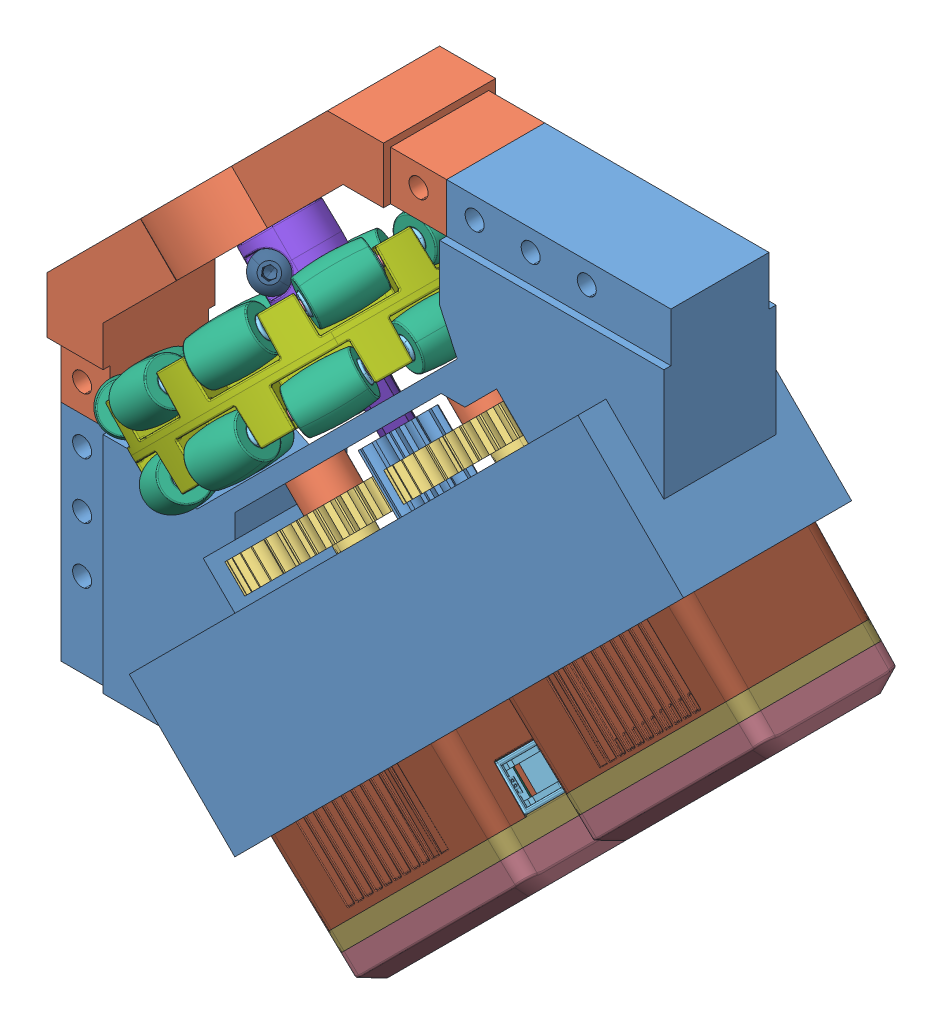
SolidWorks assembly HoloModuleAssemly1, configuration Default. Lengths in mm.
Overall size (169.7 169.56 123.95).
151 component instances, 28 part files, 46 mates.
Components (placement in the parent):
- Motor Bracket-1: Motor Bracket [Default] at (-26.4665 163.4033 98.185) size (148.89 148.89 38.1)
- Wheel Bracket-1: Wheel Bracket [Default] at (-26.4665 163.4033 98.185) size (88.9 88.9 38.1)
- Holo_Motor_Shaft-1: Holo_Motor_Shaft [Default] at (163.1236 9.787 110.8958) x (0.619089 0.619089 -0.483174) z (0.707107 -0.707107 0) size (3.28 3.28 30.48)
- Holo_Motor_Shaft-2: Holo_Motor_Shaft [Default] at (127.2026 -26.134 110.8958) x (-0.341656 -0.341656 -0.875524) z (0.707107 -0.707107 0) size (3.28 3.28 30.48)
- V5 Smart Motor (276-4840) no cap-1: V5 Smart Motor (276-4840) no cap [Default] at (47.4004 35.6548 110.885) x (0.707107 0.707107 0) z (-0.707107 0.707107 0) size (59.01 35.33 59.91)
  - V5 Smart Motor (276-4840).step-1: V5 Smart Motor (276-4840).step [Default] at origin size (59.01 35.33 59.91)
    - 276-4840-900 Rev6_Instruction.step-1: 276-4840-900 Rev6_Instruction.step [Default] at (-14.3 0 -17.2) size (52.79 15.94 38.15)
      - 276-4840-901 Rev6.step-1: 276-4840-901 Rev6.step [Default] at (10.75 -10.05 17.8) x (-1 0 0) z (0 0 1) size (49.9 1.6 38.15)
      - 276-4840-902 Rev2.step-1: 276-4840-902 Rev2.step [Default] at (31.25 -9.25 6.2) x (0 0 -1) z (0 -1 0) size (10.35 11.39 15.94)
      - 276-4840-022 Rev4.step-1: 276-4840-022 Rev4.step [Default] at (31.25 -9.25 6.2) x (0 0 -1) z (1 0 0) size (10.26 9.1 5.51)
    - 276-4840-110 Rev10_Instruction.step-1: 276-4840-110 Rev10_Instruction.step [Default] at (12.7 0 14.7) size (35.33 35.33 31.1)
      - 276-4840-061 Rev7_Ring_Gear_Fixed01 .6 Rev3.step-1: 276-4840-061 Rev7_Ring_Gear_Fixed01 .6 Rev3.step [Default] at origin size (28.79 28.39 24.6)
      - 276-4840-018 Rev6.step-1: 276-4840-018 Rev6.step [Default] at (0 0 6.7) x (-0.483174 0.875524 0) z (0 0 1) size (26 26 12.3)
      - 276-4840-059 Rev2.step-1: 276-4840-059 Rev2.step [Default] at (0 0 10.3) size (28.4 28.4 8.5)
      - 276-4840-062 Rev1.step-1: 276-4840-062 Rev1.step [Default] at (-12.1353 8.8168 12.3) x (0.956835 -0.290632 0) z (-0.290632 -0.956835 0) size (3.2 6.56 3.2)
      - 276-4840-062 Rev1.step-2: 276-4840-062 Rev1.step [Default] at (12.1353 8.8168 12.3) x (0.978427 0.206591 0) z (0.206591 -0.978427 0) size (3.2 6.56 3.2)
      - 276-4840-062 Rev1.step-3: 276-4840-062 Rev1.step [Default] at (-12.1353 -8.8168 12.3) x (0.72563 0.688086 0) z (0.688086 -0.72563 0) size (3.2 6.56 3.2)
    - 276-4840-001 Rev38.step-1: 276-4840-001 Rev38.step [Default] at origin size (57.3 33 46.9)
    - 276-4840-005 Rev27.step-1: 276-4840-005 Rev27.step [Default] at (0 0 -17.95) size (56.17 31.87 12.9)
    - 276-4840-004 Rev16.step-1: 276-4840-004 Rev16.step [Default] at (0 0 -19.2) size (56.01 31.71 9.21)
    - 276-4840-009 Rev3.step-1: 276-4840-009 Rev3.step [Default] at (25.45 13.5 15.7) x (0.19987 -0.979823 0) z (-0.979823 -0.19987 0) size (3.4 41.31 4.34)
    - 276-4840-009 Rev3.step-2: 276-4840-009 Rev3.step [Default] at (-25.45 -13.5 15.7) x (-0.998855 0.047836 0) z (0.047836 0.998855 0) size (3.4 41.31 4.34)
    - 276-4840-009 Rev3.step-3: 276-4840-009 Rev3.step [Default] at (25.45 -13.5 15.7) x (-0.975374 0.220559 0) z (0.220559 0.975374 0) size (3.4 41.31 4.34)
    - 276-4840-009 Rev3.step-4: 276-4840-009 Rev3.step [Default] at (-25.45 13.5 15.7) x (-0.922256 0.38658 0) z (0.38658 0.922256 0) size (3.4 41.31 4.34)
    - 276-4840-025 Rev19.step-1: 276-4840-025 Rev19.step [Default] at (12.7 0 -22.63) x (-0.993315 0.115437 0) z (0 0 1) size (14.82 14.83 35.18)
- V5 Smart Motor (276-4840) no cap-2: V5 Smart Motor (276-4840) no cap [Default] at (101.282 89.5364 110.885) x (-0.707107 -0.707107 0) z (-0.707107 0.707107 0) size (59.01 35.33 59.91)
  - V5 Smart Motor (276-4840).step-1: V5 Smart Motor (276-4840).step [Default] at origin size (59.01 35.33 59.91)
    - 276-4840-900 Rev6_Instruction.step-1: 276-4840-900 Rev6_Instruction.step [Default] at (-14.3 0 -17.2) size (52.79 15.94 38.15)
      - 276-4840-901 Rev6.step-1: 276-4840-901 Rev6.step [Default] at (10.75 -10.05 17.8) x (-1 0 0) z (0 0 1) size (49.9 1.6 38.15)
      - 276-4840-902 Rev2.step-1: 276-4840-902 Rev2.step [Default] at (31.25 -9.25 6.2) x (0 0 -1) z (0 -1 0) size (10.35 11.39 15.94)
      - 276-4840-022 Rev4.step-1: 276-4840-022 Rev4.step [Default] at (31.25 -9.25 6.2) x (0 0 -1) z (1 0 0) size (10.26 9.1 5.51)
    - 276-4840-110 Rev10_Instruction.step-1: 276-4840-110 Rev10_Instruction.step [Default] at (12.7 0 14.7) size (35.33 35.33 31.1)
      - 276-4840-061 Rev7_Ring_Gear_Fixed01 .6 Rev3.step-1: 276-4840-061 Rev7_Ring_Gear_Fixed01 .6 Rev3.step [Default] at origin size (28.79 28.39 24.6)
      - 276-4840-018 Rev6.step-1: 276-4840-018 Rev6.step [Default] at (0 0 6.7) x (-0.483174 0.875524 0) z (0 0 1) size (26 26 12.3)
      - 276-4840-059 Rev2.step-1: 276-4840-059 Rev2.step [Default] at (0 0 10.3) size (28.4 28.4 8.5)
      - 276-4840-062 Rev1.step-1: 276-4840-062 Rev1.step [Default] at (-12.1353 8.8168 12.3) x (0.956835 -0.290632 0) z (-0.290632 -0.956835 0) size (3.2 6.56 3.2)
      - 276-4840-062 Rev1.step-2: 276-4840-062 Rev1.step [Default] at (12.1353 8.8168 12.3) x (0.978427 0.206591 0) z (0.206591 -0.978427 0) size (3.2 6.56 3.2)
      - 276-4840-062 Rev1.step-3: 276-4840-062 Rev1.step [Default] at (-12.1353 -8.8168 12.3) x (0.72563 0.688086 0) z (0.688086 -0.72563 0) size (3.2 6.56 3.2)
    - 276-4840-001 Rev38.step-1: 276-4840-001 Rev38.step [Default] at origin size (57.3 33 46.9)
    - 276-4840-005 Rev27.step-1: 276-4840-005 Rev27.step [Default] at (0 0 -17.95) size (56.17 31.87 12.9)
    - 276-4840-004 Rev16.step-1: 276-4840-004 Rev16.step [Default] at (0 0 -19.2) size (56.01 31.71 9.21)
    - 276-4840-009 Rev3.step-1: 276-4840-009 Rev3.step [Default] at (25.45 13.5 15.7) x (0.19987 -0.979823 0) z (-0.979823 -0.19987 0) size (3.4 41.31 4.34)
    - 276-4840-009 Rev3.step-2: 276-4840-009 Rev3.step [Default] at (-25.45 -13.5 15.7) x (-0.998855 0.047836 0) z (0.047836 0.998855 0) size (3.4 41.31 4.34)
    - 276-4840-009 Rev3.step-3: 276-4840-009 Rev3.step [Default] at (25.45 -13.5 15.7) x (-0.975374 0.220559 0) z (0.220559 0.975374 0) size (3.4 41.31 4.34)
    - 276-4840-009 Rev3.step-4: 276-4840-009 Rev3.step [Default] at (-25.45 13.5 15.7) x (-0.922256 0.38658 0) z (0.38658 0.922256 0) size (3.4 41.31 4.34)
    - 276-4840-025 Rev19.step-1: 276-4840-025 Rev19.step [Default] at (12.7 0 -22.63) x (-0.993315 0.115437 0) z (0 0 1) size (14.82 14.83 35.18)
- 0.375_ ID x 0.875_ OD x 0.281_ WD (Radial Bearing) (217-3239).step-1: 0.375_ ID x 0.875_ OD x 0.281_ WD (Radial Bearing) (217-3239).step [Default] at (8.3515 128.5852 110.885) x (0.707107 -0.707107 0) z (0 0 1) size (7.14 22.23 22.23)
- 0.375_ ID x 0.875_ OD x 0.281_ WD (Radial Bearing) (217-3239).step-2: 0.375_ ID x 0.875_ OD x 0.281_ WD (Radial Bearing) (217-3239).step [Default] at (49.3241 87.6126 110.885) x (0.707107 -0.707107 0) z (0 0 1) size (7.14 22.23 22.23)
- 3.75_ High Strength Shaft (276-3524)-1: 3.75_ High Strength Shaft (276-3524) [Default] at (73.2098 63.727 110.885) x (-0.559442 -0.559442 -0.611596) z (-0.707107 0.707107 0) size (6.37 6.36 95.25)
- 0.375IDtoHSshaftInsert-1: 0.375IDtoHSshaftInsert [Default] at (13.4031 123.5336 110.885) x (0.432463 0.432463 -0.791171) z (-0.707107 0.707107 0) size (9.53 9.53 5.54)
- 0.375IDtoHSshaftInsert-2: 0.375IDtoHSshaftInsert [Default] at (49.3241 87.6126 110.885) x (-0.432463 -0.432463 0.791171) z (0.707107 -0.707107 0) size (9.53 9.53 5.54)
- 12T High Strength Metal Pinion with HS hole (276-2251)-1: 12T High Strength Metal Pinion with HS hole (276-2251) [Default] at (44.834 92.1027 110.885) x (-0.559442 -0.559442 -0.611596) z (-0.432463 -0.432463 0.791171) size (14.8 12.7 14.8)
- Shaft Collar (276-2010).step-1: Shaft Collar (276-2010).step [Default] at (23.8202 77.1955 110.885) x (0.5 0.5 -0.707107) z (0.707107 -0.707107 0) size (11 11.35 6.6)
- Shaft Collar (276-2010).step-2: Shaft Collar (276-2010).step [Default] at (59.7412 113.1165 110.885) x (0.5 0.5 -0.707107) z (0.707107 -0.707107 0) size (11 11.35 6.6)
- Holo 36T Gear (276-2169-002)-1: Holo 36T Gear (276-2169-002) [Default] at (63.9171 108.9407 110.885) x (0.677039 0.677039 0.288506) z (-0.707107 0.707107 0) size (40.08 40.08 7.94)
- Holo 36T Gear (276-2169-002)-2: Holo 36T Gear (276-2169-002) [Default] at (27.996 73.0197 110.885) x (0.007855 0.007855 0.999938) z (-0.707107 0.707107 0) size (40.08 40.08 7.94)
- 3.25_ Omni-Directional Wheel (276-3526) part-1: 3.25_ Omni-Directional Wheel (276-3526) part [Default] at (27.9894 108.9473 110.885) x (-0.559442 -0.559442 -0.611596) z (0.707107 -0.707107 0) size (90.82 89.11 34)
  - 3.25_ Omni-Directional Wheel (276-3526) .step-1: 3.25_ Omni-Directional Wheel (276-3526) .step [Default] at origin size (90.82 89.11 34)
    - Roller Assembly.step-1: Roller Assembly.step [Default] at (-0.0014 35.9575 7.1) x (0 0.963098 -0.269151) z (-1 0 0) size (14.05 14.05 18.75)
      - 276-3526-001 Rev 1.step-1: 276-3526-001 Rev 1.step [Default] at origin size (2 2 18.75)
      - 276-3526-003 Rev 1.step-1: 276-3526-003 Rev 1.step [Default] at origin size (6.15 6.15 14.2)
      - 276-3526-002 Rev 1.step-1: 276-3526-002 Rev 1.step [Default] x (0 0 1) z (-0.908956 0.416893 0) size (13.2 10.6 10.6)
    - Roller Assembly.step-2: Roller Assembly.step [Default] at (-19.4287 30.2567 7.1) x (0.421057 -0.655178 0.627258) z (-0.841254 -0.540641 0) size (14.05 14.05 18.75)
      - 276-3526-001 Rev 1.step-1: 276-3526-001 Rev 1.step [Default] at origin size (2 2 18.75)
      - 276-3526-003 Rev 1.step-1: 276-3526-003 Rev 1.step [Default] at origin size (6.15 6.15 14.2)
      - 276-3526-002 Rev 1.step-1: 276-3526-002 Rev 1.step [Default] x (0 0 1) z (-0.908956 0.416893 0) size (13.2 10.6 10.6)
    - Roller Assembly.step-3: Roller Assembly.step [Default] at (-35.5935 -5.1038 7.1) x (0.979746 0.140866 -0.142315) z (0.142315 -0.989821 0) size (14.05 14.05 18.75)
      - 276-3526-001 Rev 1.step-1: 276-3526-001 Rev 1.step [Default] at origin size (2 2 18.75)
      - 276-3526-003 Rev 1.step-1: 276-3526-003 Rev 1.step [Default] at origin size (6.15 6.15 14.2)
      - 276-3526-002 Rev 1.step-1: 276-3526-002 Rev 1.step [Default] x (0 0 1) z (-0.908956 0.416893 0) size (13.2 10.6 10.6)
    - Roller Assembly.step-4: Roller Assembly.step [Default] at (-10.1434 -34.4972 7.1) x (0.079373 0.27032 -0.959493) z (0.959493 -0.281733 0) size (14.05 14.05 18.75)
      - 276-3526-001 Rev 1.step-1: 276-3526-001 Rev 1.step [Default] at origin size (2 2 18.75)
      - 276-3526-003 Rev 1.step-1: 276-3526-003 Rev 1.step [Default] at origin size (6.15 6.15 14.2)
      - 276-3526-002 Rev 1.step-1: 276-3526-002 Rev 1.step [Default] x (0 0 1) z (-0.908956 0.416893 0) size (13.2 10.6 10.6)
    - Roller Assembly.step-5: Roller Assembly.step [Default] at (27.166 -23.5574 7.1) x (-0.355209 0.30779 -0.882662) z (0.654861 0.75575 0) size (14.05 14.05 18.75)
      - 276-3526-001 Rev 1.step-1: 276-3526-001 Rev 1.step [Default] at origin size (2 2 18.75)
      - 276-3526-003 Rev 1.step-1: 276-3526-003 Rev 1.step [Default] at origin size (6.15 6.15 14.2)
      - 276-3526-002 Rev 1.step-1: 276-3526-002 Rev 1.step [Default] x (0 0 1) z (-0.908956 0.416893 0) size (13.2 10.6 10.6)
    - Roller Assembly.step-6: Roller Assembly.step [Default] at (32.7138 14.9249 7.1) x (0.89908 0.410596 0.151875) z (-0.415415 0.909632 0) size (14.05 14.05 18.75)
      - 276-3526-001 Rev 1.step-1: 276-3526-001 Rev 1.step [Default] at origin size (2 2 18.75)
      - 276-3526-003 Rev 1.step-1: 276-3526-003 Rev 1.step [Default] at origin size (6.15 6.15 14.2)
      - 276-3526-002 Rev 1.step-1: 276-3526-002 Rev 1.step [Default] x (0 0 1) z (-0.908956 0.416893 0) size (13.2 10.6 10.6)
    - Roller Assembly.step-7: Roller Assembly.step [Default] at (19.4515 30.242 7.1) x (0.194707 0.302971 0.932898) z (-0.841254 0.540641 0) size (14.05 14.05 18.75)
      - 276-3526-001 Rev 1.step-1: 276-3526-001 Rev 1.step [Default] at origin size (2 2 18.75)
      - 276-3526-003 Rev 1.step-1: 276-3526-003 Rev 1.step [Default] at origin size (6.15 6.15 14.2)
      - 276-3526-002 Rev 1.step-1: 276-3526-002 Rev 1.step [Default] x (0 0 1) z (-0.908956 0.416893 0) size (13.2 10.6 10.6)
    - Roller Assembly.step-8: Roller Assembly.step [Default] at (-32.7025 14.9497 7.1) x (0.82743 -0.377875 0.415415) z (-0.415415 -0.909632 0) size (14.05 14.05 18.75)
      - 276-3526-001 Rev 1.step-1: 276-3526-001 Rev 1.step [Default] at origin size (2 2 18.75)
      - 276-3526-003 Rev 1.step-1: 276-3526-003 Rev 1.step [Default] at origin size (6.15 6.15 14.2)
      - 276-3526-002 Rev 1.step-1: 276-3526-002 Rev 1.step [Default] x (0 0 1) z (-0.908956 0.416893 0) size (13.2 10.6 10.6)
    - Roller Assembly.step-9: Roller Assembly.step [Default] at (-27.1838 -23.5369 7.1) x (0.578931 0.501646 -0.642799) z (0.654861 -0.75575 0) size (14.05 14.05 18.75)
      - 276-3526-001 Rev 1.step-1: 276-3526-001 Rev 1.step [Default] at origin size (2 2 18.75)
      - 276-3526-003 Rev 1.step-1: 276-3526-003 Rev 1.step [Default] at origin size (6.15 6.15 14.2)
      - 276-3526-002 Rev 1.step-1: 276-3526-002 Rev 1.step [Default] x (0 0 1) z (-0.908956 0.416893 0) size (13.2 10.6 10.6)
    - Roller Assembly.step-10: Roller Assembly.step [Default] at (10.1174 -34.5048 7.1) x (0.079373 -0.27032 -0.959493) z (0.959493 0.281733 0) size (14.05 14.05 18.75)
      - 276-3526-001 Rev 1.step-1: 276-3526-001 Rev 1.step [Default] at origin size (2 2 18.75)
      - 276-3526-003 Rev 1.step-1: 276-3526-003 Rev 1.step [Default] at origin size (6.15 6.15 14.2)
      - 276-3526-002 Rev 1.step-1: 276-3526-002 Rev 1.step [Default] x (0 0 1) z (-0.908956 0.416893 0) size (13.2 10.6 10.6)
    - Roller Assembly.step-11: Roller Assembly.step [Default] at (35.5896 -5.1307 7.1) x (0.988515 -0.142127 -0.05136) z (0.142315 0.989821 0) size (14.05 14.05 18.75)
      - 276-3526-001 Rev 1.step-1: 276-3526-001 Rev 1.step [Default] at origin size (2 2 18.75)
      - 276-3526-003 Rev 1.step-1: 276-3526-003 Rev 1.step [Default] at origin size (6.15 6.15 14.2)
      - 276-3526-002 Rev 1.step-1: 276-3526-002 Rev 1.step [Default] x (0 0 1) z (-0.908956 0.416893 0) size (13.2 10.6 10.6)
    - Roller Assembly.step-12: Roller Assembly.step [Default] at (10.1434 34.4972 -7.1) x (0.083119 0.283078 -0.955489) z (0.959493 -0.281733 0) size (14.05 14.05 18.75)
      - 276-3526-001 Rev 1.step-1: 276-3526-001 Rev 1.step [Default] at origin size (2 2 18.75)
      - 276-3526-003 Rev 1.step-1: 276-3526-003 Rev 1.step [Default] at origin size (6.15 6.15 14.2)
      - 276-3526-002 Rev 1.step-1: 276-3526-002 Rev 1.step [Default] x (0 0 1) z (-0.908956 0.416893 0) size (13.2 10.6 10.6)
    - Roller Assembly.step-13: Roller Assembly.step [Default] at (27.1838 23.5369 -7.1) x (0.582526 0.504762 -0.637086) z (0.654861 -0.75575 0) size (14.05 14.05 18.75)
      - 276-3526-001 Rev 1.step-1: 276-3526-001 Rev 1.step [Default] at origin size (2 2 18.75)
      - 276-3526-003 Rev 1.step-1: 276-3526-003 Rev 1.step [Default] at origin size (6.15 6.15 14.2)
      - 276-3526-002 Rev 1.step-1: 276-3526-002 Rev 1.step [Default] x (0 0 1) z (-0.908956 0.416893 0) size (13.2 10.6 10.6)
    - Roller Assembly.step-14: Roller Assembly.step [Default] at (35.5935 5.1038 -7.1) x (0.926341 0.133188 -0.352355) z (0.142315 -0.989821 0) size (14.05 14.05 18.75)
      - 276-3526-001 Rev 1.step-1: 276-3526-001 Rev 1.step [Default] at origin size (2 2 18.75)
      - 276-3526-003 Rev 1.step-1: 276-3526-003 Rev 1.step [Default] at origin size (6.15 6.15 14.2)
      - 276-3526-002 Rev 1.step-1: 276-3526-002 Rev 1.step [Default] x (0 0 1) z (-0.908956 0.416893 0) size (13.2 10.6 10.6)
    - Roller Assembly.step-15: Roller Assembly.step [Default] at (32.7025 -14.9497 -7.1) x (0.897398 -0.409828 0.163453) z (-0.415415 -0.909632 0) size (14.05 14.05 18.75)
      - 276-3526-001 Rev 1.step-1: 276-3526-001 Rev 1.step [Default] at origin size (2 2 18.75)
      - 276-3526-003 Rev 1.step-1: 276-3526-003 Rev 1.step [Default] at origin size (6.15 6.15 14.2)
      - 276-3526-002 Rev 1.step-1: 276-3526-002 Rev 1.step [Default] x (0 0 1) z (-0.908956 0.416893 0) size (13.2 10.6 10.6)
    - Roller Assembly.step-16: Roller Assembly.step [Default] at (19.4287 -30.2567 -7.1) x (0.277612 -0.431972 0.858098) z (-0.841254 -0.540641 0) size (14.05 14.05 18.75)
      - 276-3526-001 Rev 1.step-1: 276-3526-001 Rev 1.step [Default] at origin size (2 2 18.75)
      - 276-3526-003 Rev 1.step-1: 276-3526-003 Rev 1.step [Default] at origin size (6.15 6.15 14.2)
      - 276-3526-002 Rev 1.step-1: 276-3526-002 Rev 1.step [Default] x (0 0 1) z (-0.908956 0.416893 0) size (13.2 10.6 10.6)
    - Roller Assembly.step-17: Roller Assembly.step [Default] at (-0.0136 -35.9575 -7.1) x (0 -0.239919 0.970793) z (-1 0 0) size (14.05 14.05 18.75)
      - 276-3526-001 Rev 1.step-1: 276-3526-001 Rev 1.step [Default] at origin size (2 2 18.75)
      - 276-3526-003 Rev 1.step-1: 276-3526-003 Rev 1.step [Default] at origin size (6.15 6.15 14.2)
      - 276-3526-002 Rev 1.step-1: 276-3526-002 Rev 1.step [Default] x (0 0 1) z (-0.908956 0.416893 0) size (13.2 10.6 10.6)
    - Roller Assembly.step-18: Roller Assembly.step [Default] at (-19.4515 -30.242 -7.1) x (0.31008 0.482494 0.819176) z (-0.841254 0.540641 0) size (14.05 14.05 18.75)
      - 276-3526-001 Rev 1.step-1: 276-3526-001 Rev 1.step [Default] at origin size (2 2 18.75)
      - 276-3526-003 Rev 1.step-1: 276-3526-003 Rev 1.step [Default] at origin size (6.15 6.15 14.2)
      - 276-3526-002 Rev 1.step-1: 276-3526-002 Rev 1.step [Default] x (0 0 1) z (-0.908956 0.416893 0) size (13.2 10.6 10.6)
    - Roller Assembly.step-19: Roller Assembly.step [Default] at (-32.7138 -14.9249 -7.1) x (0.58758 0.268339 0.763377) z (-0.415415 0.909632 0) size (14.05 14.05 18.75)
      - 276-3526-001 Rev 1.step-1: 276-3526-001 Rev 1.step [Default] at origin size (2 2 18.75)
      - 276-3526-003 Rev 1.step-1: 276-3526-003 Rev 1.step [Default] at origin size (6.15 6.15 14.2)
      - 276-3526-002 Rev 1.step-1: 276-3526-002 Rev 1.step [Default] x (0 0 1) z (-0.908956 0.416893 0) size (13.2 10.6 10.6)
    - Roller Assembly.step-20: Roller Assembly.step [Default] at (-35.5896 5.1307 -7.1) x (0.965498 -0.138818 0.220323) z (0.142315 0.989821 0) size (14.05 14.05 18.75)
      - 276-3526-001 Rev 1.step-1: 276-3526-001 Rev 1.step [Default] at origin size (2 2 18.75)
      - 276-3526-003 Rev 1.step-1: 276-3526-003 Rev 1.step [Default] at origin size (6.15 6.15 14.2)
      - 276-3526-002 Rev 1.step-1: 276-3526-002 Rev 1.step [Default] x (0 0 1) z (-0.908956 0.416893 0) size (13.2 10.6 10.6)
    - Roller Assembly.step-21: Roller Assembly.step [Default] at (-27.166 23.5574 -7.1) x (0.75327 -0.652712 -0.080935) z (0.654861 0.75575 0) size (14.05 14.05 18.75)
      - 276-3526-001 Rev 1.step-1: 276-3526-001 Rev 1.step [Default] at origin size (2 2 18.75)
      - 276-3526-003 Rev 1.step-1: 276-3526-003 Rev 1.step [Default] at origin size (6.15 6.15 14.2)
      - 276-3526-002 Rev 1.step-1: 276-3526-002 Rev 1.step [Default] x (0 0 1) z (-0.908956 0.416893 0) size (13.2 10.6 10.6)
    - Roller Assembly.step-22: Roller Assembly.step [Default] at (-10.1174 34.5048 -7.1) x (0.123782 -0.421563 -0.898311) z (0.959493 0.281733 0) size (14.05 14.05 18.75)
      - 276-3526-001 Rev 1.step-1: 276-3526-001 Rev 1.step [Default] at origin size (2 2 18.75)
      - 276-3526-003 Rev 1.step-1: 276-3526-003 Rev 1.step [Default] at origin size (6.15 6.15 14.2)
      - 276-3526-002 Rev 1.step-1: 276-3526-002 Rev 1.step [Default] x (0 0 1) z (-0.908956 0.416893 0) size (13.2 10.6 10.6)
    - 276-3526-004 Rev 1.step-1: 276-3526-004 Rev 1.step [Default] at origin size (78.5 78.5 19.07)
- Clamping Shaft Collar (276-3891).step-1: Clamping Shaft Collar (276-3891).step [Default] at (17.8932 119.0435 110.885) x (0.5 0.5 0.707107) z (-0.707107 0.707107 0) size (17.85 18.85 12.92)
  - 276-3891-001 Rev1.step-1: 276-3891-001 Rev1.step [Default] at origin size (15.89 15.86 12.7)
  - 276-1027-001.step-1: 276-1027-001.step [Default] at (-2.788 -4.7 0) x (0 0.866025 -0.5) z (0 0.5 0.866025) size (8.61 4.98 9.94)
  - 276-1004-001_SBS0832-0500SS.step-1: 276-1004-001_SBS0832-0500SS.step [Default] at (4.9978 -4.7 0) x (-1 0 0) z (0 0.924225 0.381849) size (14.91 7.92 7.92)
Mates (geometry in assembly coordinates):
- Coincident1: coincident anti-aligned: plane of Motor Bracket-1 through (62.4335 163.4033 123.585) normal (-1 0 0); plane of Wheel Bracket-1 through (62.4335 163.4033 123.585) normal (1 0 0)
- Coincident2: coincident anti-aligned: plane of Motor Bracket-1 through (-26.4665 74.5033 123.585) normal (0 1 0); plane of Wheel Bracket-1 through (-26.4665 74.5033 123.585) normal (0 -1 0)
- Coincident3: coincident aligned: plane of Motor Bracket-1 through (-26.4665 163.4033 123.585) normal (0 0 1); plane of Wheel Bracket-1 through (-26.4665 163.4033 123.585) normal (0 0 1)
- Coincident4: coincident anti-aligned: plane of Motor Bracket-1 through (42.8761 69.3142 125.7566) normal (0.707107 -0.707107 0); plane of V5 Smart Motor (276-4840) no cap-1/V5 Smart Motor (276-4840).step-1/276-4840-110 Rev10_Instruction.step-1/276-4840-059 Rev2.step-1 through (37.2888 63.727 110.885) normal (-0.707107 0.707107 0)
- Coincident5: coincident anti-aligned: plane of Holo_Motor_Shaft-2 through (40.9922 60.0764 110.8958) normal (0.707107 -0.707107 0); plane of V5 Smart Motor (276-4840) no cap-1/V5 Smart Motor (276-4840).step-1/276-4840-110 Rev10_Instruction.step-1/276-4840-018 Rev6.step-1 through (40.9657 60.05 110.885) normal (-0.707107 0.707107 0)
- Coincident6: coincident anti-aligned: plane of Holo_Motor_Shaft-2 through (234.5253 -134.3375 113.0527) normal (0.341656 0.341656 0.875524); plane of V5 Smart Motor (276-4840) no cap-1/V5 Smart Motor (276-4840).step-1/276-4840-110 Rev10_Instruction.step-1/276-4840-018 Rev6.step-1 through (36.8407 63.2789 113.0793) normal (-0.341656 -0.341656 -0.875524)
- Coincident7: coincident anti-aligned: plane of Holo_Motor_Shaft-2 through (236.4909 -132.3719 111.5186) normal (0.619089 0.619089 -0.483174); plane of V5 Smart Motor (276-4840) no cap-1/V5 Smart Motor (276-4840).step-1/276-4840-110 Rev10_Instruction.step-1/276-4840-018 Rev6.step-1 through (38.8404 65.2786 111.5186) normal (-0.619089 -0.619089 0.483174)
- Concentric2: concentric aligned: circle of Motor Bracket-1; circle of V5 Smart Motor (276-4840) no cap-1/V5 Smart Motor (276-4840).step-1/276-4840-001 Rev38.step-1
- Concentric3: concentric anti-aligned: circle of Motor Bracket-1; circle of V5 Smart Motor (276-4840) no cap-1/V5 Smart Motor (276-4840).step-1/276-4840-110 Rev10_Instruction.step-1/276-4840-059 Rev2.step-1
- Coincident11: coincident anti-aligned: plane of Holo_Motor_Shaft-1 through (76.9132 95.9974 110.8958) normal (0.707107 -0.707107 0); plane of V5 Smart Motor (276-4840) no cap-2/V5 Smart Motor (276-4840).step-1/276-4840-110 Rev10_Instruction.step-1/276-4840-018 Rev6.step-1 through (76.8868 95.971 110.885) normal (-0.707107 0.707107 0)
- Coincident12: coincident anti-aligned: plane of Holo_Motor_Shaft-1 through (270.4463 -98.4165 113.0527) normal (0.341656 0.341656 0.875524); plane of V5 Smart Motor (276-4840) no cap-2/V5 Smart Motor (276-4840).step-1/276-4840-110 Rev10_Instruction.step-1/276-4840-018 Rev6.step-1 through (74.7614 101.1996 111.5186) normal (-0.341656 -0.341656 -0.875524)
- Coincident13: coincident anti-aligned: plane of Holo_Motor_Shaft-1 through (271.3271 -97.5357 108.7389) normal (0.619089 0.619089 -0.483174); plane of V5 Smart Motor (276-4840) no cap-2/V5 Smart Motor (276-4840).step-1/276-4840-110 Rev10_Instruction.step-1/276-4840-018 Rev6.step-1 through (73.6579 100.096 108.6907) normal (-0.619089 -0.619089 0.483174)
- Coincident14: coincident anti-aligned: plane of Motor Bracket-1 through (80.5162 106.9544 121.4784) normal (0.707107 -0.707107 0); plane of V5 Smart Motor (276-4840) no cap-2/V5 Smart Motor (276-4840).step-1/276-4840-110 Rev10_Instruction.step-1/276-4840-059 Rev2.step-1 through (73.2098 99.648 110.885) normal (-0.707107 0.707107 0)
- Concentric4: concentric aligned: circle of Motor Bracket-1; circle of V5 Smart Motor (276-4840) no cap-2/V5 Smart Motor (276-4840).step-1/276-4840-110 Rev10_Instruction.step-1/276-4840-059 Rev2.step-1
- Concentric5: concentric aligned: circle of Motor Bracket-1; circle of V5 Smart Motor (276-4840) no cap-2/V5 Smart Motor (276-4840).step-1/276-4840-001 Rev38.step-1
- Concentric6: concentric anti-aligned: cylinder of Motor Bracket-1 through (49.3241 87.6126 110.885) axis (0.707107 -0.707107 0) radius 11.1125; cylinder of 0.375_ ID x 0.875_ OD x 0.281_ WD (Radial Bearing) (217-3239).step-2 through (39.045 97.8918 110.885) axis (-0.707107 0.707107 0) radius 11.113
- Coincident17: coincident aligned: plane of Motor Bracket-1 through (49.3241 87.6126 123.585) normal (-0.707107 0.707107 0); plane of 0.375_ ID x 0.875_ OD x 0.281_ WD (Radial Bearing) (217-3239).step-2 through (45.6734 83.9618 110.885) normal (-0.707107 0.707107 0)
- Concentric7: concentric aligned: cylinder of Wheel Bracket-1 through (13.4031 123.5336 110.885) axis (-0.707107 0.707107 0) radius 11.1125; cylinder of 0.375_ ID x 0.875_ OD x 0.281_ WD (Radial Bearing) (217-3239).step-1 through (-1.9276 138.8644 110.885) axis (-0.707107 0.707107 0) radius 11.113
- Coincident18: coincident aligned: plane of Wheel Bracket-1 through (13.4031 123.5336 123.585) normal (0.707107 -0.707107 0); plane of 0.375_ ID x 0.875_ OD x 0.281_ WD (Radial Bearing) (217-3239).step-1 through (8.901 119.0315 110.885) normal (0.707107 -0.707107 0)
- Concentric9: concentric anti-aligned: cylinder of 0.375_ ID x 0.875_ OD x 0.281_ WD (Radial Bearing) (217-3239).step-1 through (-1.9276 138.8644 110.885) axis (-0.707107 0.707107 0) radius 4.763; cylinder of 0.375IDtoHSshaftInsert-1 through (9.4877 127.449 110.885) axis (0.707107 -0.707107 0) radius 4.7625
- Coincident22: coincident aligned: plane of 0.375_ ID x 0.875_ OD x 0.281_ WD (Radial Bearing) (217-3239).step-1 through (8.901 119.0315 110.885) normal (0.707107 -0.707107 0); plane of 0.375IDtoHSshaftInsert-1 through (13.4031 123.5336 110.885) normal (0.707107 -0.707107 0)
- Coincident23: coincident aligned: plane of 0.375_ ID x 0.875_ OD x 0.281_ WD (Radial Bearing) (217-3239).step-2 through (45.6734 83.9618 110.885) normal (-0.707107 0.707107 0); plane of 0.375IDtoHSshaftInsert-2 through (49.3241 87.6126 110.885) normal (-0.707107 0.707107 0)
- Concentric10: concentric aligned: cylinder of 0.375_ ID x 0.875_ OD x 0.281_ WD (Radial Bearing) (217-3239).step-2 through (39.045 97.8918 110.885) axis (-0.707107 0.707107 0) radius 4.763; cylinder of 0.375IDtoHSshaftInsert-2 through (53.2395 83.6972 110.885) axis (-0.707107 0.707107 0) radius 4.7625
- Coincident25: coincident aligned: plane of Motor Bracket-1 through (73.2098 63.727 98.185) normal (0.707107 -0.707107 0); plane of 3.75_ High Strength Shaft (276-3524)-1 through (73.2098 63.727 110.885) normal (0.707107 -0.707107 0)
- Coincident30: coincident anti-aligned: plane of 3.75_ High Strength Shaft (276-3524)-1 through (-145.0034 276.5661 110.6094) normal (-0.559442 -0.559442 -0.611596); plane of 0.375IDtoHSshaftInsert-1 through (6.5581 124.5194 111.0532) normal (0.559442 0.559442 0.611596)
- Coincident31: coincident anti-aligned: plane of 3.75_ High Strength Shaft (276-3524)-1 through (-142.5112 279.0582 114.685) normal (-0.432463 -0.432463 0.791171); plane of 0.375IDtoHSshaftInsert-1 through (6.6226 124.5839 111.7658) normal (0.432463 0.432463 -0.791171)
- Coincident32: coincident anti-aligned: plane of 3.75_ High Strength Shaft (276-3524)-1 through (-139.765 281.8044 109.6611) normal (0.432463 0.432463 -0.791171); plane of 0.375IDtoHSshaftInsert-2 through (53.1206 83.5783 106.7419) normal (-0.432463 -0.432463 0.791171)
- Coincident33: coincident anti-aligned: plane of 3.75_ High Strength Shaft (276-3524)-1 through (-145.0034 276.5661 110.6094) normal (-0.559442 -0.559442 -0.611596); plane of 0.375IDtoHSshaftInsert-2 through (52.6167 83.0744 106.8331) normal (0.559442 0.559442 0.611596)
- Coincident43: coincident anti-aligned: plane of Motor Bracket-1 through (49.3241 87.6126 123.585) normal (-0.707107 0.707107 0); plane of 12T High Strength Metal Pinion with HS hole (276-2251)-1 through (47.6073 85.8958 112.7337) normal (0.707107 -0.707107 0)
- Coincident44: coincident anti-aligned: plane of 3.75_ High Strength Shaft (276-3524)-1 through (-145.0034 276.5661 110.6094) normal (-0.559442 -0.559442 -0.611596); plane of 12T High Strength Metal Pinion with HS hole (276-2251)-1 through (33.371 102.32 106.8331) normal (0.559442 0.559442 0.611596)
- Coincident45: coincident anti-aligned: plane of 3.75_ High Strength Shaft (276-3524)-1 through (-142.5112 279.0582 114.685) normal (-0.432463 -0.432463 0.791171); plane of 12T High Strength Metal Pinion with HS hole (276-2251)-1 through (34.1128 103.0618 115.0281) normal (0.432463 0.432463 -0.791171)
- Coincident47: coincident anti-aligned: plane of Motor Bracket-1 through (39.4459 97.4909 123.585) normal (0.707107 -0.707107 0); plane of Shaft Collar (276-2010).step-2 through (57.4064 115.4514 110.885) normal (-0.707107 0.707107 0)
- Concentric11: concentric aligned: circle of Motor Bracket-1; circle of Shaft Collar (276-2010).step-2
- Coincident48: coincident anti-aligned: plane of Motor Bracket-1 through (39.4459 97.4909 123.585) normal (0.707107 -0.707107 0); plane of Shaft Collar (276-2010).step-1 through (21.4854 79.5304 110.885) normal (-0.707107 0.707107 0)
- Concentric12: concentric aligned: circle of Motor Bracket-1; circle of Shaft Collar (276-2010).step-1
- Concentric13: concentric aligned: circle of Motor Bracket-1; circle of Holo 36T Gear (276-2169-002)-1
- Coincident51: coincident anti-aligned: plane of Motor Bracket-1 through (49.3241 87.6126 123.585) normal (-0.707107 0.707107 0); plane of Holo 36T Gear (276-2169-002)-1 through (67.2847 105.5731 110.885) normal (0.707107 -0.707107 0)
- Coincident52: coincident anti-aligned: plane of Motor Bracket-1 through (49.3241 87.6126 123.585) normal (-0.707107 0.707107 0); plane of Holo 36T Gear (276-2169-002)-2 through (31.3636 69.6521 110.885) normal (0.707107 -0.707107 0)
- Concentric15: concentric aligned: circle of Motor Bracket-1; circle of Holo 36T Gear (276-2169-002)-2
- Coincident53: coincident anti-aligned: plane of 3.75_ High Strength Shaft (276-3524)-1 through (-142.5112 279.0582 114.685) normal (-0.432463 -0.432463 0.791171); plane of 3.25_ Omni-Directional Wheel (276-3526) part-1/3.25_ Omni-Directional Wheel (276-3526) .step-1/276-3526-004 Rev 1.step-1 through (21.6574 116.0857 115.3388) normal (0.432463 0.432463 -0.791171)
- Coincident54: coincident anti-aligned: plane of 3.75_ High Strength Shaft (276-3524)-1 through (-141.4509 280.1185 114.4931) normal (0.559442 0.559442 0.611596); plane of 3.25_ Omni-Directional Wheel (276-3526) part-1/3.25_ Omni-Directional Wheel (276-3526) .step-1/276-3526-004 Rev 1.step-1 through (24.4035 118.8318 110.3148) normal (-0.559442 -0.559442 -0.611596)
- Distance3: distance = 6.35 mm anti-aligned: plane of 3.25_ Omni-Directional Wheel (276-3526) part-1/3.25_ Omni-Directional Wheel (276-3526) .step-1/276-3526-004 Rev 1.step-1 through (32.4796 104.4572 110.885) normal (0.707107 -0.707107 0); plane of Motor Bracket-1 through (36.9697 99.9671 123.585) normal (-0.707107 0.707107 0)
- GearMate3: gear = 25.4 : 76.2 mm: cylinder of Holo 36T Gear (276-2169-002)-2 through (42.9059 83.4394 114.2626) axis (0.707107 -0.707107 0) radius 2.9504; cylinder of 12T High Strength Metal Pinion with HS hole (276-2251)-1 through (49.1211 87.4096 116.9815) axis (-0.707107 0.707107 0) radius 3
- GearMate4: gear = 5.9009 : 5.9009 mm: cylinder of Holo 36T Gear (276-2169-002)-2 through (38.1842 78.7177 96.5317) axis (0.707107 -0.707107 0) radius 2.9504; cylinder of Holo 36T Gear (276-2169-002)-1 through (63.5011 104.0347 93.0513) axis (0.707107 -0.707107 0) radius 2.9504
- Coincident57: coincident anti-aligned: plane of Wheel Bracket-1 through (13.4031 123.5336 123.585) normal (0.707107 -0.707107 0); plane of Clamping Shaft Collar (276-3891).step-1/276-3891-001 Rev1.step-1 through (13.4031 123.5336 110.885) normal (-0.707107 0.707107 0)
- Concentric17: concentric aligned: circle of Wheel Bracket-1; circle of Clamping Shaft Collar (276-3891).step-1/276-3891-001 Rev1.step-1
